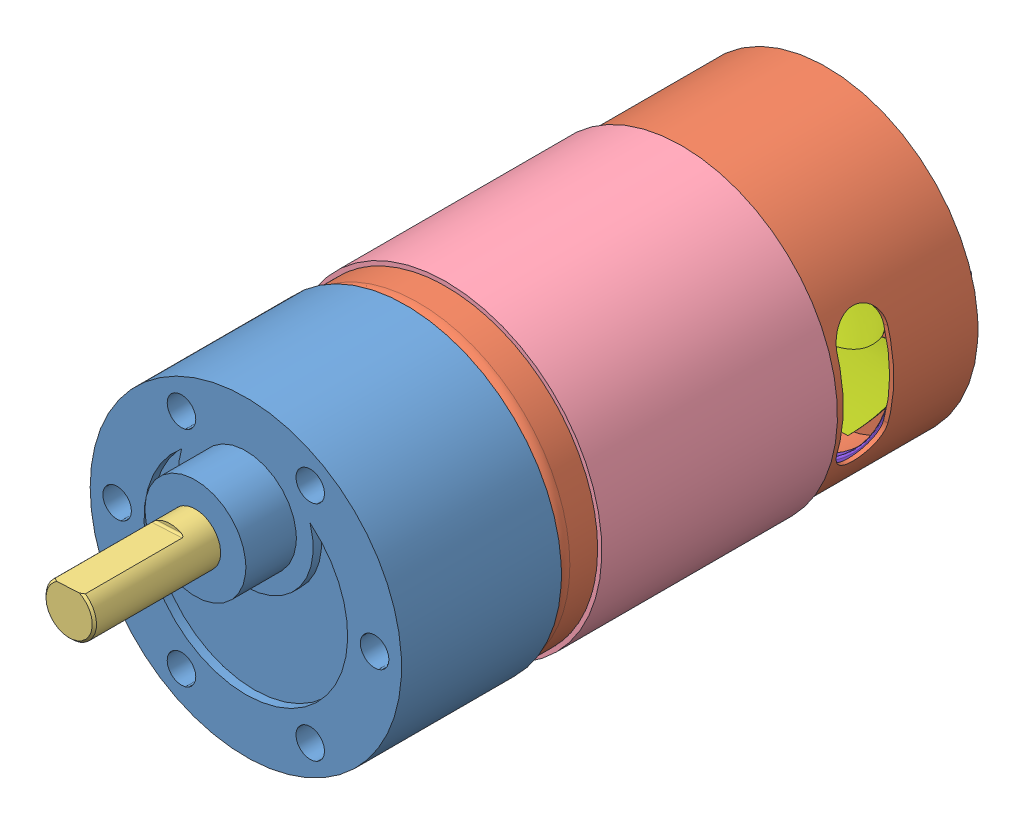
SolidWorks assembly Motor JGB37-545, configuration Predeterminado. Lengths in mm.
Overall size (37 37 94.88).
11 component instances, 11 part files, 33 mates.
Components (placement in the parent):
- Reduction box body-1: Reduction box body [Default] at (-12.375 1.5 54.875)
- Motor body-1: Motor body [Predeterminado] at (-12.375 1.5 4.875)
- Shaft-1: Shaft [Predeterminado] at (-12.375 8.5 67.775) x (0.998724 0.050497 0) z (0 0 1)
- Cover-1: Cover [Predeterminado] at (-12.375 1.5 22.075)
- Rotor-1: Rotor [Predeterminado] at (-12.375 1.5 32.275) x (0.999981 -0.006201 0) z (0 0 1)
- Magnets-1: Magnets [Default] at (-12.375 1.5 22.875) x (0 1 0) z (0 0 1)
- Fan-1: Fan [Default] at (-12.375 1.5 12.975) x (0.995635 -0.093332 0) z (0.093332 0.995635 0)
- Terminals-1: Terminals [Default] at (-12.375 1.5 5.375) x (1 0 0) z (0 0 -1)
- Gear 1-1: Gear 1 [Default] at (-12.375 1.5 62.275) x (-0.006201 -0.999981 0) z (0.999981 -0.006201 0)
- Gear 2-1: Gear 2 [Default] at (-12.375 -3.65 64.275) x (-0.919431 0.393252 0) z (-0.393252 -0.919431 0)
- Gear 3-1: Gear 3 [Default] at (-12.375 8.5 66.275) x (0.050497 -0.998724 0) z (0.998724 0.050497 0)
Mates (geometry in assembly coordinates):
- Coincidente1: coincident anti-aligned: plane of Reduction box body-1 through (-12.375 1.5 54.875) normal (0 0 -1); plane of Motor body-1 through (-12.375 1.5 54.875) normal (0 0 1)
- Concéntrica1: concentric aligned: cylinder of Reduction box body-1 through (-12.375 1.5 73.875) axis (0 0 -1) radius 18.5; cylinder of Motor body-1 through (-12.375 1.5 54.875) axis (0 0 -1) radius 18
- Distancia1: distance = 15 mm aligned: plane of Shaft-1 through (-12.375 8.5 94.875) normal (0 0 1); plane of GM37-3525_HT_Motor-1 through (-12.375 8.5 79.875) normal (0 0 1)
- Concéntrica2: concentric anti-aligned: cylinder of Reduction box body-1 through (-12.375 8.5 54.874) axis (0 0 1) radius 3; cylinder of Shaft-1 through (-12.375 8.5 94.875) axis (0 0 -1) radius 3
- Distancia2: distance = 4.8 mm anti-aligned: plane of Cover-1 through (-12.375 1.5 50.075) normal (0 0 1); plane of GM37-3525_HT_Motor-1 through (-12.375 1.5 54.875) normal (0 0 -1)
- Concéntrica3: concentric aligned: cylinder of Motor body-1 through (-12.375 1.5 54.875) axis (0 0 -1) radius 18; cylinder of Cover-1 through (-12.375 1.5 50.075) axis (0 0 -1) radius 18
- Concentric1: concentric aligned: cylinder of Motor body-1 through (-12.375 1.5 54.875) axis (0 0 -1) radius 17.5; cylinder of Rotor-1 through (-12.375 1.5 30.875) axis (0 0 -1) radius 13
- Distance1: distance = 4 mm aligned: plane of Rotor-1 through (-15.3249 1.5183 8.875) normal (0 0 -1); plane of Motor-1 through (-12.375 1.5 4.875) normal (0 0 -1)
- Concentric3: concentric aligned: cylinder of Motor body-1 through (-12.375 1.5 54.875) axis (0 0 -1) radius 17.5; cylinder of Magnets-1 through (-12.375 1.5 42.875) axis (0 0 -1) radius 14.5
- Distance4: distance = 2 mm aligned: plane of magnets-1 through (-12.375 1.5 22.875) normal (0 0 -1); plane of Rotor-1 through (-12.375 1.5 24.875) normal (0 0 -1)
- Parallel2: parallel aligned: plane of Magnets-1 through (1.2357 6.5 42.875) normal (1 0 0)
- Coincident9: coincident anti-aligned: plane of Rotor-1 through (-12.375 1.5 9.375) normal (0.999981 -0.006201 0); plane of Fan-1 through (-12.3567 4.4499 14.0996) normal (-0.999981 0.006201 0)
- Concentric5: concentric aligned: cylinder of Rotor-1 through (-12.375 1.5 62.275) axis (0 0 -1) radius 2; cylinder of Fan-1 through (-12.375 1.5 8.7004) axis (0 0 -1) radius 2
- Distance5: distance = 2 mm anti-aligned: plane of Rotor-1 through (-14.5478 4.2211 14.975) normal (0 0 -1); plane of Fan-1 through (-12.375 1.5 12.975) normal (0 0 1)
- Coincident13: coincident anti-aligned: plane of Motor body-1 through (-25.125 -0.5 15.375) normal (0 1 0); plane of Terminals-1 through (-25.125 -0.5 4.875) normal (0 -1 0)
- Coincident14: coincident anti-aligned: plane of Motor body-1 through (0.375 3.5 15.375) normal (-1 0 0); plane of Terminals-1 through (0.375 -0.5 4.875) normal (1 0 0)
- Coincident15: coincident aligned: plane of Motor body-1 through (-12.375 -16 5.875) normal (0 0 1); plane of Terminals-1 through (-12.375 1.5 5.875) normal (0 0 1)
- Coincident16: coincident anti-aligned: plane of Terminals-1 through (-25.125 0.9005 0) normal (0 0 -1)
- Coincident17: coincident aligned: plane of Terminals-1 through (0 3 6.875) normal (1 0 0)
- Coincident18: coincident anti-aligned: plane of Terminals-1 through (-0.75 0 6.875) normal (0 -1 0)
- Parallel3: parallel anti-aligned: plane of Cover-1 through (-9.275 -16.231 50.075) normal (-1 0 0)
- Parallel4: parallel aligned: plane of Reduction box body-1 through (-18.625 -12.75 55.025) normal (1 0 0)
- Concentric6: concentric anti-aligned: cylinder of Rotor-1 through (-12.375 1.5 62.275) axis (0 0 -1) radius 2; cylinder of Gear 1-1 through (-12.375 1.5 60.275) axis (0 0 1) radius 2
- Coincident19: coincident anti-aligned: plane of Rotor-1 through (-12.3657 3 56.275) normal (0.006201 0.999981 0); plane of Gear 1-1 through (-12.3657 3 60.275) normal (-0.006201 -0.999981 0)
- Coincident26: coincident aligned: plane of Rotor-1 through (-12.375 1.5 62.275) normal (0 0 1); plane of Gear 1-1 through (-12.375 1.5 62.275) normal (0 0 1)
- Concentric7: concentric anti-aligned: cylinder of Shaft-1 through (-12.375 8.5 94.875) axis (0 0 -1) radius 3; cylinder of Gear 5-1 through (-12.375 8.5 64.275) axis (0 0 1) radius 5
- Coincident23: coincident anti-aligned: plane of Shaft-1 through (-12.4129 9.249 70.275) normal (0.050497 -0.998724 0); plane of Gear 5-1 through (-12.4129 9.249 67.775) normal (-0.050497 0.998724 0)
- Coincident24: coincident anti-aligned: plane of Shaft-1 through (-12.375 8.5 70.275) normal (0 0 -1); plane of Gear 5-1 through (-12.375 8.5 70.275) normal (0 0 1)
- Parallel5: parallel anti-aligned: plane of Shaft-1 through (-12.375 8.5 94.875) normal (0 0 1); plane of Gear 2-1 through (-12.375 -3.65 58.275) normal (0 0 -1)
- Coincident27: coincident aligned: plane of Gear 1-1 through (-12.375 1.5 60.275) normal (0 0 -1); plane of Gear 2-1 through (-12.375 -3.65 60.275) normal (0 0 -1)
- Concentric9: concentric aligned: cylinder of Reduction box body-1 through (-12.375 -3.65 65.875) axis (0 0 1) radius 2; cylinder of Gear 2-1 through (-12.375 -3.65 58.275) axis (0 0 1) radius 1
- GearMate2: gear = 28 : 23 mm: cylinder of Gear 2-1 through (-12.375 -3.65 60.275) axis (0 0 1) radius 2.5; cylinder of Gear 1-1 through (-12.375 1.5 60.275) axis (0 0 1) radius 3
- GearMate3: gear = 23 : 100 mm: cylinder of Gear 2-1 through (-12.375 -3.65 64.275) axis (0 0 -1) radius 10; cylinder of Gear 3-1 through (-12.375 8.5 62.275) axis (0 0 1) radius 2.5
